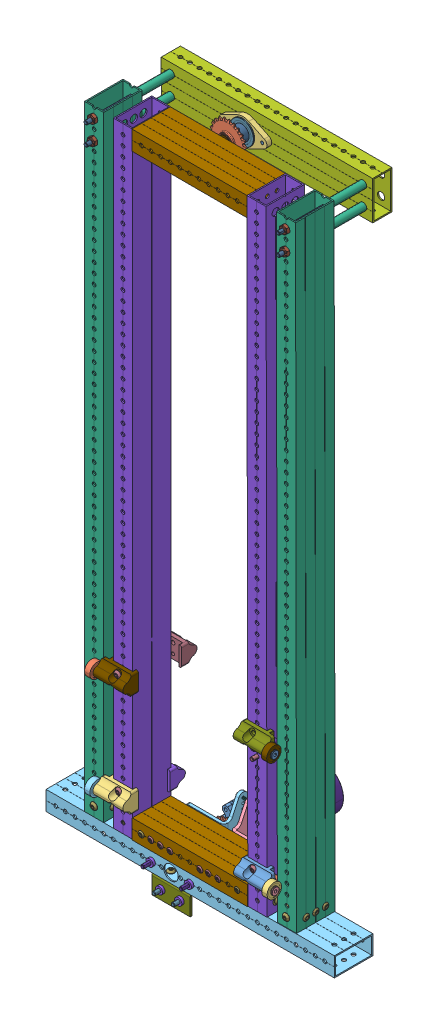
SolidWorks assembly WCP - GreyT Elevator (Cascade, 1 Stage).step, configuration Default. Lengths in mm. (continued)
Components (placement in the parent): (continued)
- WCP-0379 Rev1^WCP - GreyT Elevator (Cascade, 1 Stage).step-4: WCP-0379 Rev1^WCP - GreyT Elevator (Cascade, 1 Stage).step [Default] at (-127 22.225 0) x (0 0 -1) z (1 0 0) size (47.24 20.64 21.84) (virtual)
- WCP-0374 Rev1^WCP - GreyT Elevator (Cascade, 1 Stage).step-4: WCP-0374 Rev1^WCP - GreyT Elevator (Cascade, 1 Stage).step [Default] at (-127 22.225 0) x (0 0 -1) z (1 0 0) size (44.07 19.05 18.67) (virtual)
- 10-32 BHCS - No Thread_WCP-0252 - 0.375^WCP - GreyT Elevator (Cascade, 1 Stage).step-30: 10-32 BHCS - No Thread_WCP-0252 - 0.375^WCP - GreyT Elevator (Cascade, 1 Stage).step [Default] at (-127 11.1125 -12.7) x (-0.583861 0 0.811854) z (0.811854 0 0.583861) size (9.17 12.1 9.17) (virtual)
- 10-32 BHCS - No Thread_WCP-0252 - 0.375^WCP - GreyT Elevator (Cascade, 1 Stage).step-31: 10-32 BHCS - No Thread_WCP-0252 - 0.375^WCP - GreyT Elevator (Cascade, 1 Stage).step [Default] at (-127 11.1125 0) x (-0.583861 0 0.811854) z (0.811854 0 0.583861) size (9.17 12.1 9.17) (virtual)
- 10-32 BHCS - No Thread_WCP-0252 - 0.375^WCP - GreyT Elevator (Cascade, 1 Stage).step-32: 10-32 BHCS - No Thread_WCP-0252 - 0.375^WCP - GreyT Elevator (Cascade, 1 Stage).step [Default] at (-127 11.1125 12.7) x (-0.583861 0 0.811854) z (0.811854 0 0.583861) size (9.17 12.1 9.17) (virtual)
- WCP-0207 Rev1^WCP - GreyT Elevator (Cascade, 1 Stage).step-3: WCP-0207 Rev1^WCP - GreyT Elevator (Cascade, 1 Stage).step [Default] at (-127 812.8 -50.5828) x (0 0 -1) z (0.999873 0.015939 0) size (50.8 9.5 9.5) (virtual)
- WCP-0207 Rev1^WCP - GreyT Elevator (Cascade, 1 Stage).step-4: WCP-0207 Rev1^WCP - GreyT Elevator (Cascade, 1 Stage).step [Default] at (-126.9354 787.4001 -50.5828) x (0 0 -1) z (0.999873 0.015939 0) size (50.8 9.5 9.5) (virtual)
- 10-32 BHCS - No Thread_WCP-0252 - 0.375^WCP - GreyT Elevator (Cascade, 1 Stage).step-33: 10-32 BHCS - No Thread_WCP-0252 - 0.375^WCP - GreyT Elevator (Cascade, 1 Stage).step [Default] at (-127 25.4 25.4) x (-0.238233 -0.971208 0) z (-0.971208 0.238233 0) size (9.17 12.1 9.17) (virtual)
- 10-32 BHCS - No Thread_WCP-0252 - 0.375^WCP - GreyT Elevator (Cascade, 1 Stage).step-34: 10-32 BHCS - No Thread_WCP-0252 - 0.375^WCP - GreyT Elevator (Cascade, 1 Stage).step [Default] at (-127 25.4 -25.4) x (-0.705419 -0.708791 0) z (0.708791 -0.705419 0) size (9.17 12.1 9.17) (virtual)
- WCP-EX-0018-003^WCP - GreyT Elevator (Cascade, 1 Stage).step-2: WCP-EX-0018-003^WCP - GreyT Elevator (Cascade, 1 Stage).step [Default] at (-88.9 127 0) x (0 1 0) z (1 0 0) size (812.8 50.8 25.4) (virtual)
- 10-32 BHCS - No Thread_WCP-0261 - 2.500^WCP - GreyT Elevator (Cascade, 1 Stage).step-11: 10-32 BHCS - No Thread_WCP-0261 - 2.500^WCP - GreyT Elevator (Cascade, 1 Stage).step [Default] at (-88.9 63.5 30.1625) x (-0.238233 -0.971208 0) z (-0.971208 0.238233 0) size (9.17 66.07 9.17) (virtual)
- 10-32 BHCS - No Thread_WCP-0261 - 2.500^WCP - GreyT Elevator (Cascade, 1 Stage).step-12: 10-32 BHCS - No Thread_WCP-0261 - 2.500^WCP - GreyT Elevator (Cascade, 1 Stage).step [Default] at (-88.9 50.8 -30.1625) x (-0.035589 0.999367 0) z (-0.999367 -0.035589 0) size (9.17 66.07 9.17) (virtual)
- 10-32 BHCS - No Thread_WCP-0261 - 2.500^WCP - GreyT Elevator (Cascade, 1 Stage).step-13: 10-32 BHCS - No Thread_WCP-0261 - 2.500^WCP - GreyT Elevator (Cascade, 1 Stage).step [Default] at (-88.8365 198.4231 32.0651) x (-0.238233 -0.971208 0) z (-0.971208 0.238233 0) size (9.17 66.07 9.17) (virtual)
- 10-32 BHCS - No Thread_WCP-0261 - 2.500^WCP - GreyT Elevator (Cascade, 1 Stage).step-14: 10-32 BHCS - No Thread_WCP-0261 - 2.500^WCP - GreyT Elevator (Cascade, 1 Stage).step [Default] at (-88.8365 185.7231 -30.1625) x (-0.035589 0.999367 0) z (-0.999367 -0.035589 0) size (9.17 66.07 9.17) (virtual)
- 10-32 BHCS - No Thread_WCP-0252 - 0.375^WCP - GreyT Elevator (Cascade, 1 Stage).step-35: 10-32 BHCS - No Thread_WCP-0252 - 0.375^WCP - GreyT Elevator (Cascade, 1 Stage).step [Default] at (-77.7875 25.4 -12.7) x (0 0.635714 0.771925) z (0 -0.771925 0.635714) size (9.17 12.1 9.17) (virtual)
- 10-32 BHCS - No Thread_WCP-0252 - 0.375^WCP - GreyT Elevator (Cascade, 1 Stage).step-36: 10-32 BHCS - No Thread_WCP-0252 - 0.375^WCP - GreyT Elevator (Cascade, 1 Stage).step [Default] at (-77.7875 25.4 0) x (0 0.635714 0.771925) z (0 -0.771925 0.635714) size (9.17 12.1 9.17) (virtual)
- 10-32 BHCS - No Thread_WCP-0252 - 0.375^WCP - GreyT Elevator (Cascade, 1 Stage).step-37: 10-32 BHCS - No Thread_WCP-0252 - 0.375^WCP - GreyT Elevator (Cascade, 1 Stage).step [Default] at (-77.7875 25.4 12.7) x (0 0.635714 0.771925) z (0 -0.771925 0.635714) size (9.17 12.1 9.17) (virtual)
- 10-32 BHCS - No Thread_WCP-0252 - 0.375^WCP - GreyT Elevator (Cascade, 1 Stage).step-38: 10-32 BHCS - No Thread_WCP-0252 - 0.375^WCP - GreyT Elevator (Cascade, 1 Stage).step [Default] at (-63.5 25.4 25.4) x (-0.238233 -0.971208 0) z (-0.971208 0.238233 0) size (9.17 12.1 9.17) (virtual)
- WCP-0374 Rev1^WCP - GreyT Elevator (Cascade, 1 Stage).step-5: WCP-0374 Rev1^WCP - GreyT Elevator (Cascade, 1 Stage).step [Default] at (-66.675 25.4 0) x (0 0 -1) z (0 -1 0) size (44.07 19.05 18.67) (virtual)
- WCP-0379 Rev1^WCP - GreyT Elevator (Cascade, 1 Stage).step-5: WCP-0379 Rev1^WCP - GreyT Elevator (Cascade, 1 Stage).step [Default] at (-66.675 25.4 0) x (0 0 -1) z (0 -1 0) size (47.24 20.64 21.84) (virtual)
- 10-32 BHCS - No Thread_WCP-0252 - 0.375^WCP - GreyT Elevator (Cascade, 1 Stage).step-39: 10-32 BHCS - No Thread_WCP-0252 - 0.375^WCP - GreyT Elevator (Cascade, 1 Stage).step [Default] at (-63.5 25.4 -25.4) x (-0.705419 -0.708791 0) z (0.708791 -0.705419 0) size (9.17 12.1 9.17) (virtual)
- 10-32 BHCS - No Thread_WCP-0252 - 0.375^WCP - GreyT Elevator (Cascade, 1 Stage).step-40: 10-32 BHCS - No Thread_WCP-0252 - 0.375^WCP - GreyT Elevator (Cascade, 1 Stage).step [Default] at (-88.7441 24.976 -25.2488) x (-0.705419 -0.708791 0) z (0.708791 -0.705419 0) size (9.17 12.1 9.17) (virtual)
- 10-32 BHCS - No Thread_WCP-0252 - 0.375^WCP - GreyT Elevator (Cascade, 1 Stage).step-41: 10-32 BHCS - No Thread_WCP-0252 - 0.375^WCP - GreyT Elevator (Cascade, 1 Stage).step [Default] at (-72.5907 24.976 -1.6268) x (0 0.635714 0.771925) z (0 -0.771925 0.635714) size (9.17 12.1 9.17) (virtual)
- 10-32 BHCS - No Thread_WCP-0252 - 0.375^WCP - GreyT Elevator (Cascade, 1 Stage).step-42: 10-32 BHCS - No Thread_WCP-0252 - 0.375^WCP - GreyT Elevator (Cascade, 1 Stage).step [Default] at (-72.5907 24.976 11.0732) x (0 0.635714 0.771925) z (0 -0.771925 0.635714) size (9.17 12.1 9.17) (virtual)
- 10-32 BHCS - No Thread_WCP-0252 - 0.375^WCP - GreyT Elevator (Cascade, 1 Stage).step-43: 10-32 BHCS - No Thread_WCP-0252 - 0.375^WCP - GreyT Elevator (Cascade, 1 Stage).step [Default] at (-72.4033 24.976 -14.3268) x (0 0.635714 0.771925) z (0 -0.771925 0.635714) size (9.17 12.1 9.17) (virtual)
- 10-32 BHCS - No Thread_WCP-0252 - 0.375^WCP - GreyT Elevator (Cascade, 1 Stage).step-44: 10-32 BHCS - No Thread_WCP-0252 - 0.375^WCP - GreyT Elevator (Cascade, 1 Stage).step [Default] at (-88.7441 24.976 21.9952) x (-0.238233 -0.971208 0) z (-0.971208 0.238233 0) size (9.17 12.1 9.17) (virtual)
- WCP-0379 Rev1^WCP - GreyT Elevator (Cascade, 1 Stage).step-6: WCP-0379 Rev1^WCP - GreyT Elevator (Cascade, 1 Stage).step [Default] at (-91.9191 24.849 -1.6268) x (0 0 -1) z (0 -1 0) size (47.24 20.64 21.84) (virtual)
- WCP-0374 Rev1^WCP - GreyT Elevator (Cascade, 1 Stage).step-6: WCP-0374 Rev1^WCP - GreyT Elevator (Cascade, 1 Stage).step [Default] at (-91.9191 24.976 -1.6268) x (0 0 -1) z (0 -1 0) size (44.07 19.05 18.67) (virtual)
- WCP-0583-027 Rev1^WCP - GreyT Elevator (Cascade, 1 Stage).step-1: WCP-0583-027 Rev1^WCP - GreyT Elevator (Cascade, 1 Stage).step [Default] at (-38.1 -12.7 25.4) x (0 -1 0) z (1 0 0) size (25.4 25.4 50.8) (virtual)
- REV-21-1650-V1.1.step-1: REV-21-1650-V1.1.step [Default] at (-25.4 0 -115.5875) size (68.13 68.01 93.35)
- REV-21-2102-4-1-cartridge-1: REV-21-2102-4-1-cartridge [Default] at (-25.4 0 -90.2375) size (61.91 50.8 16.85)
- REV-21-2104-hex-socket-output-1: REV-21-2104-hex-socket-output [Default] at (-25.4 0 -74.4125) x (0 0 1) z (-1 0 0) size (23.2 50.8 61.92)
- REV-21-2106-universal-input-1: REV-21-2106-universal-input [Default] at (-25.4 0 -106.0625) size (61.91 50.8 19.05)
- 1_500_L_10_thru_WCP-0205-2: 1_500_L_10_thru_WCP-0205 [Default] at (12.7 0 -43.561) x (0 0 1) z (-0.94684 -0.321705 0) size (38.1 9.5 9.5)
- 1_500_L_10_thru_WCP-0205-3: 1_500_L_10_thru_WCP-0205 [Default] at (-63.5 0 -43.561) x (0 0 1) z (-0.860119 0.510093 0) size (38.1 9.5 9.5)
- Part4^WCP - GreyT Elevator (Cascade, 1 Stage).step-1: Part4^WCP - GreyT Elevator (Cascade, 1 Stage).step [Default] at (-25.4 0 -64.8875) (virtual)
Mates (geometry in assembly coordinates):
- Coincident1: coincident aligned: plane of WCP-EX-0018-005^WCP - GreyT Elevator (Cascade, 1 Stage).step-1 through (126.705 826.1491 0.0759) normal (-0.001569 0.999999 0.000005); plane of WCP-EX-0018-003^WCP - GreyT Elevator (Cascade, 1 Stage).step-1 through (88.6027 826.0894 1.0044) normal (-0.001569 0.999999 0.000005)
- Distance2: distance = 12.7 mm anti-aligned: plane of WCP-EX-0018-003^WCP - GreyT Elevator (Cascade, 1 Stage).step-1 through (101.7227 597.5098 -24.3659) normal (0.999996 0.001569 0.002419); plane of WCP-EX-0018-005^WCP - GreyT Elevator (Cascade, 1 Stage).step-1 through (115.2188 13.33 25.4412) normal (-0.999996 -0.001569 -0.002419)
- Coincident13: coincident anti-aligned: plane of WCP-EX-0018-002^WCP - GreyT Elevator (Cascade, 1 Stage).step-1 through (139.796 775.3781 -75.9828) normal (0 0 1); circle of WCP-0207 Rev1^WCP - GreyT Elevator (Cascade, 1 Stage).step-3
- Distance9: distance = 6.3627 mm aligned: plane of WCP-0326 Rev1^WCP - GreyT Elevator (Cascade, 1 Stage).step-12 through (-126.9354 787.4001 30.367) normal (0 0 1); plane of 10-32 SHCS - No Thread_WCP-0274 - 4.500^WCP - GreyT Elevator (Cascade, 1 Stage).step-4 through (-126.9354 787.4001 36.7297) normal (0 0 1)
- Distance10: distance = 6.3627 mm aligned: plane of WCP-0326 Rev1^WCP - GreyT Elevator (Cascade, 1 Stage).step-2 through (126.9992 813.4457 30.367) normal (0 0 1); plane of 10-32 SHCS - No Thread_WCP-0274 - 4.500^WCP - GreyT Elevator (Cascade, 1 Stage).step-2 through (126.9992 813.4457 36.7297) normal (0 0 1)
- Distance11: distance = 6.3627 mm aligned: plane of WCP-0326 Rev1^WCP - GreyT Elevator (Cascade, 1 Stage).step-1 through (127.0637 788.0458 30.367) normal (0 0 1); plane of 10-32 SHCS - No Thread_WCP-0274 - 4.500^WCP - GreyT Elevator (Cascade, 1 Stage).step-1 through (127.0637 788.0458 36.7297) normal (0 0 1)
- Concentric2: concentric anti-aligned: circle of WCP-0326 Rev1^WCP - GreyT Elevator (Cascade, 1 Stage).step-12; circle of 10-32 SHCS - No Thread_WCP-0274 - 4.500^WCP - GreyT Elevator (Cascade, 1 Stage).step-4
- Concentric4: concentric anti-aligned: circle of 10-32 SHCS - No Thread_WCP-0274 - 4.500^WCP - GreyT Elevator (Cascade, 1 Stage).step-2; circle of WCP-0326 Rev1^WCP - GreyT Elevator (Cascade, 1 Stage).step-2
- Concentric5: concentric anti-aligned: circle of WCP-0326 Rev1^WCP - GreyT Elevator (Cascade, 1 Stage).step-11; circle of 10-32 SHCS - No Thread_WCP-0274 - 4.500^WCP - GreyT Elevator (Cascade, 1 Stage).step-3
- Concentric9: concentric anti-aligned: cylinder of 10-32 SHCS - No Thread_WCP-0274 - 4.500^WCP - GreyT Elevator (Cascade, 1 Stage).step-3 through (-127 812.8 36.7297) axis (0 0 -1) radius 2.413; cylinder of WCP-0207 Rev1^WCP - GreyT Elevator (Cascade, 1 Stage).step-3 through (-127 812.8 -75.9828) axis (0 0 1) radius 2.4892
- Concentric10: concentric anti-aligned: cylinder of 10-32 SHCS - No Thread_WCP-0274 - 4.500^WCP - GreyT Elevator (Cascade, 1 Stage).step-4 through (-126.9354 787.4001 36.7297) axis (0 0 -1) radius 2.413; cylinder of WCP-0207 Rev1^WCP - GreyT Elevator (Cascade, 1 Stage).step-4 through (-126.9354 787.4001 -75.9828) axis (0 0 1) radius 2.4892
- Concentric11: concentric anti-aligned: cylinder of 10-32 SHCS - No Thread_WCP-0274 - 4.500^WCP - GreyT Elevator (Cascade, 1 Stage).step-2 through (126.9992 813.4457 36.7297) axis (0 0 -1) radius 2.413; cylinder of WCP-0207 Rev1^WCP - GreyT Elevator (Cascade, 1 Stage).step-1 through (126.9992 813.4457 -75.9828) axis (0 0 1) radius 2.4892
- Concentric12: concentric anti-aligned: cylinder of 10-32 SHCS - No Thread_WCP-0274 - 4.500^WCP - GreyT Elevator (Cascade, 1 Stage).step-1 through (127.0637 788.0458 36.7297) axis (0 0 -1) radius 2.413; cylinder of WCP-0207 Rev1^WCP - GreyT Elevator (Cascade, 1 Stage).step-2 through (127.0637 788.0458 -75.9828) axis (0 0 1) radius 2.4892
- Concentric13: concentric aligned: circle of 10-32 SHCS - No Thread_WCP-0274 - 4.500^WCP - GreyT Elevator (Cascade, 1 Stage).step-1; circle of WCP-0326 Rev1^WCP - GreyT Elevator (Cascade, 1 Stage).step-1
- Concentric14: concentric anti-aligned: circle of WCP-EX-0018-002^WCP - GreyT Elevator (Cascade, 1 Stage).step-1; circle of WCP-0207 Rev1^WCP - GreyT Elevator (Cascade, 1 Stage).step-4
- Concentric15: concentric anti-aligned: circle of WCP-EX-0018-002^WCP - GreyT Elevator (Cascade, 1 Stage).step-1; circle of WCP-0207 Rev1^WCP - GreyT Elevator (Cascade, 1 Stage).step-2
- Concentric16: concentric anti-aligned: circle of WCP-EX-0018-002^WCP - GreyT Elevator (Cascade, 1 Stage).step-1; circle of WCP-0207 Rev1^WCP - GreyT Elevator (Cascade, 1 Stage).step-1
- Concentric17: concentric anti-aligned: circle of WCP-EX-0018-002^WCP - GreyT Elevator (Cascade, 1 Stage).step-1; circle of WCP-0207 Rev1^WCP - GreyT Elevator (Cascade, 1 Stage).step-3
- Concentric18: concentric anti-aligned: cylinder of 10-32 BHCS - No Thread_WCP-0257 - 1.500.step-1 through (0.0319 800.4229 -69.6328) axis (0 0 -1) radius 2.3749; cylinder of WCP-0476 Rev1^WCP - GreyT Elevator (Cascade, 1 Stage).step-2 through (0.0319 800.4229 -69.6328) axis (0 0 1) radius 2.0193
- Concentric19: concentric anti-aligned: cylinder of 10-32 BHCS - No Thread_WCP-0257 - 1.500.step-2 through (-50.768 800.2938 -69.6328) axis (0 0 -1) radius 2.3749; cylinder of WCP-0476 Rev1^WCP - GreyT Elevator (Cascade, 1 Stage).step-2 through (-50.768 800.2938 -69.6328) axis (0 0 1) radius 2.0193
- Concentric20: concentric anti-aligned: cylinder of 10-32 BHCS - No Thread_WCP-0257 - 1.500.step-2 through (-50.768 800.2938 -69.6328) axis (0 0 -1) radius 2.3749; cylinder of WCP-0476 Rev1^WCP - GreyT Elevator (Cascade, 1 Stage).step-3 through (-50.768 800.2938 -101.3828) axis (0 0 1) radius 2.0193
- Coincident38: coincident anti-aligned: plane of 10-32 BHCS - No Thread_WCP-0257 - 1.500.step-1 through (0.0319 800.4229 -107.7328) normal (0 0 1); plane of WCP-0476 Rev1^WCP - GreyT Elevator (Cascade, 1 Stage).step-3 through (-25.368 800.2938 -107.7328) normal (0 0 -1)
- Coincident39: coincident anti-aligned: plane of 10-32 BHCS - No Thread_WCP-0257 - 1.500.step-2 through (-50.768 800.2938 -107.7328) normal (0 0 1); plane of WCP-0476 Rev1^WCP - GreyT Elevator (Cascade, 1 Stage).step-3 through (-25.368 800.2938 -107.7328) normal (0 0 -1)
- Concentric24: concentric anti-aligned: cylinder of WCP-EX-0018-002^WCP - GreyT Elevator (Cascade, 1 Stage).step-1 through (126.9992 813.4457 -75.9818) axis (0 0 -1) radius 4.7625; cylinder of WCP-0207 Rev1^WCP - GreyT Elevator (Cascade, 1 Stage).step-1 through (126.9992 813.4457 -75.9828) axis (0 0 1) radius 4.7498
- Concentric25: concentric anti-aligned: cylinder of WCP-EX-0018-002^WCP - GreyT Elevator (Cascade, 1 Stage).step-1 through (127.0637 788.0458 -75.9818) axis (0 0 -1) radius 4.7625; cylinder of WCP-0207 Rev1^WCP - GreyT Elevator (Cascade, 1 Stage).step-2 through (127.0637 788.0458 -75.9828) axis (0 0 1) radius 4.7498
- Coincident41: coincident anti-aligned: plane of WCP-EX-0018-002^WCP - GreyT Elevator (Cascade, 1 Stage).step-1 through (139.796 775.3781 -75.9828) normal (0 0 1); plane of WCP-0207 Rev1^WCP - GreyT Elevator (Cascade, 1 Stage).step-2 through (127.0637 788.0458 -75.9828) normal (0 0 -1)
- Coincident42: coincident anti-aligned: plane of WCP-EX-0018-002^WCP - GreyT Elevator (Cascade, 1 Stage).step-1 through (139.796 775.3781 -75.9828) normal (0 0 1); plane of WCP-0207 Rev1^WCP - GreyT Elevator (Cascade, 1 Stage).step-1 through (126.9992 813.4457 -75.9828) normal (0 0 -1)
- Coincident43: coincident anti-aligned: plane of WCP-EX-0018-002^WCP - GreyT Elevator (Cascade, 1 Stage).step-1 through (139.7314 800.778 -77.5703) normal (0 0 -1); plane of 10-32 SHCS - No Thread_WCP-0274 - 4.500^WCP - GreyT Elevator (Cascade, 1 Stage).step-4 through (-126.9354 787.4001 -77.5703) normal (0 0 1)
- Concentric26: concentric anti-aligned: cylinder of WCP-0476 Rev1^WCP - GreyT Elevator (Cascade, 1 Stage).step-2 through (-25.368 800.3583 -69.6328) axis (0 0 -1) radius 14.2875; cylinder of WCP-0785_0_500_flanged_thunderhex_bearing.step-3 through (-25.368 800.3583 -18.7651) axis (0 0 1) radius 14.2875
- Concentric27: concentric aligned: circle of WCP-0790_500L_500_hex.step-1; cylinder of WCP-0785_0_500_flanged_thunderhex_bearing.step-3 through (-25.368 800.3583 -18.7651) axis (0 0 1) radius 6.875
- Coincident44: coincident anti-aligned: plane of WCP-0599 Rev1^WCP - GreyT Elevator (Cascade, 1 Stage).step-1 through (-26.1223 793.9249 -109.3203) normal (-0.128795 -0.991671 0); plane of WCP-0790_500L_500_hex.step-1 through (-29.9106 794.4169 -55.3453) normal (0.128795 0.991671 0)
- Coincident45: coincident anti-aligned: plane of WCP-0599 Rev1^WCP - GreyT Elevator (Cascade, 1 Stage).step-1 through (-20.2716 796.3603 -109.3203) normal (0.794415 -0.607376 0); plane of WCP-0790_500L_500_hex.step-1 through (-22.4939 793.4536 -55.3453) normal (-0.794415 0.607376 0)
- Coincident46: coincident anti-aligned: plane of WCP-0560 Rev1^WCP - GreyT Elevator (Cascade, 1 Stage).step-2 through (-22.4939 793.4536 -45.8203) normal (0.128795 0.991671 0); plane of WCP-0599 Rev1^WCP - GreyT Elevator (Cascade, 1 Stage).step-1 through (-26.1223 793.9249 -109.3203) normal (-0.128795 -0.991671 0)
- Coincident47: coincident anti-aligned: plane of WCP-0560 Rev1^WCP - GreyT Elevator (Cascade, 1 Stage).step-2 through (-18.0226 799.3019 -45.8203) normal (-0.794415 0.607376 0); plane of WCP-0599 Rev1^WCP - GreyT Elevator (Cascade, 1 Stage).step-1 through (-20.2716 796.3603 -109.3203) normal (0.794415 -0.607376 0)
- Concentric28: concentric anti-aligned: circle of WCP-0571 Rev1^WCP - GreyT Elevator (Cascade, 1 Stage).step-1; circle of WCP-0599 Rev1^WCP - GreyT Elevator (Cascade, 1 Stage).step-1
- Coincident49: coincident aligned: plane of WCP-0560 Rev1^WCP - GreyT Elevator (Cascade, 1 Stage).step-2 through (-25.323 800.25 -45.8203) normal (0 0 1); plane of WCP-0599 Rev1^WCP - GreyT Elevator (Cascade, 1 Stage).step-1 through (-25.3061 800.2094 -45.8203) normal (0 0 1)
- Coincident50: coincident anti-aligned: plane of WCP-0571 Rev1^WCP - GreyT Elevator (Cascade, 1 Stage).step-1 through (-25.3061 795.6247 -45.8203) normal (0 0 -1); plane of WCP-0560 Rev1^WCP - GreyT Elevator (Cascade, 1 Stage).step-2 through (-25.323 800.25 -45.8203) normal (0 0 1)
- Concentric29: concentric anti-aligned: cylinder of WCP-EX-0018-002^WCP - GreyT Elevator (Cascade, 1 Stage).step-1 through (-50.768 800.2938 -75.9828) axis (0 0 -1) radius 2.4892; cylinder of WCP-0476 Rev1^WCP - GreyT Elevator (Cascade, 1 Stage).step-2 through (-50.768 800.2938 -69.6328) axis (0 0 1) radius 2.0193
- Concentric30: concentric anti-aligned: cylinder of WCP-EX-0018-002^WCP - GreyT Elevator (Cascade, 1 Stage).step-1 through (0.0319 800.4229 -75.9828) axis (0 0 -1) radius 2.4892; cylinder of WCP-0476 Rev1^WCP - GreyT Elevator (Cascade, 1 Stage).step-2 through (0.0319 800.4229 -69.6328) axis (0 0 1) radius 2.0193
- Coincident51: coincident anti-aligned: plane of WCP-0560 Rev1^WCP - GreyT Elevator (Cascade, 1 Stage).step-2 through (-25.323 800.25 -55.3453) normal (0 0 -1); plane of WCP-0790_500L_500_hex.step-1 through (-25.368 800.3583 -55.3453) normal (0 0 1)
- Concentric31: concentric aligned: circle of WCP-0571 Rev1^WCP - GreyT Elevator (Cascade, 1 Stage).step-2; circle of WCP-0599 Rev1^WCP - GreyT Elevator (Cascade, 1 Stage).step-1
- Concentric32: concentric anti-aligned: circle of WCP-0476 Rev1^WCP - GreyT Elevator (Cascade, 1 Stage).step-3; circle of WCP-0785_0_500_flanged_thunderhex_bearing.step-2
- Coincident55: coincident anti-aligned: plane of WCP-0476 Rev1^WCP - GreyT Elevator (Cascade, 1 Stage).step-2 through (-25.368 800.3583 -69.6328) normal (0 0 1); plane of WCP-0785_0_500_flanged_thunderhex_bearing.step-3 through (-36.1398 809.7445 -69.6328) normal (0 0 -1)
- Coincident56: coincident anti-aligned: plane of WCP-0790_500L_500_hex.step-1 through (-25.368 800.3583 -68.0453) normal (0 0 -1); plane of WCP-0785_0_500_flanged_thunderhex_bearing.step-3 through (-32.6073 806.6664 -68.0453) normal (0 0 1)
- Coincident57: coincident anti-aligned: plane of WCP-EX-0018-002^WCP - GreyT Elevator (Cascade, 1 Stage).step-1 through (139.796 775.3781 -75.9828) normal (0 0 1); plane of WCP-0476 Rev1^WCP - GreyT Elevator (Cascade, 1 Stage).step-2 through (-25.368 800.3583 -75.9828) normal (0 0 -1)
- Coincident58: coincident anti-aligned: plane of WCP-EX-0018-002^WCP - GreyT Elevator (Cascade, 1 Stage).step-1 through (139.796 775.3781 -101.3828) normal (0 0 -1); plane of WCP-0476 Rev1^WCP - GreyT Elevator (Cascade, 1 Stage).step-3 through (-25.368 800.2938 -101.3828) normal (0 0 1)
- Coincident59: coincident anti-aligned: plane of WCP-0476 Rev1^WCP - GreyT Elevator (Cascade, 1 Stage).step-3 through (-25.368 800.2938 -107.7328) normal (0 0 -1); plane of WCP-0785_0_500_flanged_thunderhex_bearing.step-2 through (-19.5771 813.3551 -107.7328) normal (0 0 1)
- Coincident60: coincident anti-aligned: plane of WCP-0571 Rev1^WCP - GreyT Elevator (Cascade, 1 Stage).step-2 through (-24.6727 795.6687 -109.3203) normal (0 0 1); plane of WCP-0599 Rev1^WCP - GreyT Elevator (Cascade, 1 Stage).step-1 through (-25.3061 800.2094 -109.3203) normal (0 0 -1)
- Distance12: distance = 6.5799 mm aligned: plane of WCP-0326 Rev1^WCP - GreyT Elevator (Cascade, 1 Stage).step-11 through (-127 812.8 30.1498) normal (0 0 1); plane of 10-32 SHCS - No Thread_WCP-0274 - 4.500^WCP - GreyT Elevator (Cascade, 1 Stage).step-3 through (-127 812.8 36.7297) normal (0 0 1)
- Coincident69: coincident anti-aligned: plane of WCP-EX-0018-002^WCP - GreyT Elevator (Cascade, 1 Stage).step-1 through (139.796 775.3781 -75.9828) normal (0 0 1); plane of WCP-0207 Rev1^WCP - GreyT Elevator (Cascade, 1 Stage).step-4 through (-126.9354 787.4001 -75.9828) normal (0 0 -1)
- Coincident70: coincident anti-aligned: plane of WCP-EX-0018-002^WCP - GreyT Elevator (Cascade, 1 Stage).step-1 through (139.7314 800.778 -77.5703) normal (0 0 -1); plane of 10-32 SHCS - No Thread_WCP-0274 - 4.500^WCP - GreyT Elevator (Cascade, 1 Stage).step-3 through (-127 812.8 -77.5703) normal (0 0 1)
- Coincident71: coincident aligned: plane of 10-32 SHCS - No Thread_WCP-0274 - 4.500^WCP - GreyT Elevator (Cascade, 1 Stage).step-1 through (127.0637 788.0458 36.7297) normal (0 0 1); plane of 10-32 SHCS - No Thread_WCP-0274 - 4.500^WCP - GreyT Elevator (Cascade, 1 Stage).step-2 through (126.9992 813.4457 36.7297) normal (0 0 1)
- Coincident72: coincident aligned: plane of 10-32 SHCS - No Thread_WCP-0274 - 4.500^WCP - GreyT Elevator (Cascade, 1 Stage).step-3 through (-127 812.8 36.7297) normal (0 0 1); plane of 10-32 SHCS - No Thread_WCP-0274 - 4.500^WCP - GreyT Elevator (Cascade, 1 Stage).step-4 through (-126.9354 787.4001 36.7297) normal (0 0 1)
- Coincident80: coincident anti-aligned: plane of WCP-EX-0018-005^WCP - GreyT Elevator (Cascade, 1 Stage).step-2 through (-114.3 12.7 25.4) normal (0 0 1); plane of WCP-0326 Rev1^WCP - GreyT Elevator (Cascade, 1 Stage).step-11 through (-127 812.8 25.4) normal (0 0 -1)
- Concentric33: concentric aligned: circle of WCP-EX-0018-005^WCP - GreyT Elevator (Cascade, 1 Stage).step-2; circle of 10-32 SHCS - No Thread_WCP-0274 - 4.500^WCP - GreyT Elevator (Cascade, 1 Stage).step-3
- Coincident81: coincident anti-aligned: plane of WCP-EX-0018-003^WCP - GreyT Elevator (Cascade, 1 Stage).step-1 through (76.3228 597.4699 -24.4273) normal (-0.999996 -0.001569 -0.002419); plane of WCP-EX-0018-004^WCP - GreyT Elevator (Cascade, 1 Stage).step-2 through (75.9226 813.3695 0.9736) normal (0.999996 0.001569 0.002419)
- Coincident82: coincident aligned: plane of WCP-EX-0018-003^WCP - GreyT Elevator (Cascade, 1 Stage).step-1 through (88.6027 826.0894 1.0044) normal (-0.001569 0.999999 0.000005); plane of WCP-EX-0018-004^WCP - GreyT Elevator (Cascade, 1 Stage).step-2 through (75.8413 826.0692 26.3736) normal (-0.001569 0.999999 0.000005)
- Coincident83: coincident aligned: plane of WCP-EX-0018-003^WCP - GreyT Elevator (Cascade, 1 Stage).step-1 through (76.1999 597.4695 26.3725) normal (-0.002419 -0.000009 0.999997); plane of WCP-EX-0018-004^WCP - GreyT Elevator (Cascade, 1 Stage).step-2 through (75.8413 826.0692 26.3736) normal (-0.002419 -0.000009 0.999997)
- Coincident84: coincident anti-aligned: plane of WCP-0323 - Elevator Clamping Block-7^WCP - GreyT Elevator (Cascade, 1 Stage).step-1/WCP-0323-001 Rev2(6)^WCP-0323 - Elevator Clamping Block-7_WCP - GreyT Elevator (Cascade, 1 Stage).step-1 through (-101.6 192.0731 20.892) normal (1 0 0); plane of WCP-EX-0018-003^WCP - GreyT Elevator (Cascade, 1 Stage).step-2 through (-101.6 241.3 -25.4) normal (-1 0 0)
- Coincident85: coincident anti-aligned: plane of WCP-0323 - Elevator Clamping Block-7^WCP - GreyT Elevator (Cascade, 1 Stage).step-1/WCP-0323-001 Rev2(6)^WCP-0323 - Elevator Clamping Block-7_WCP - GreyT Elevator (Cascade, 1 Stage).step-1 through (-101.6 192.0731 25.4) normal (0 0 -1); plane of WCP-EX-0018-003^WCP - GreyT Elevator (Cascade, 1 Stage).step-2 through (-76.2 241.3 25.4) normal (0 0 1)
- Concentric49: concentric aligned: cylinder of WCP-0323 - Elevator Clamping Block-7^WCP - GreyT Elevator (Cascade, 1 Stage).step-1/WCP-0323-001 Rev2(6)^WCP-0323 - Elevator Clamping Block-7_WCP - GreyT Elevator (Cascade, 1 Stage).step-1 through (-88.8365 185.7231 41.275) axis (0 0 -1) radius 2.4892; cylinder of 10-32 BHCS - No Thread_WCP-0261 - 2.500^WCP - GreyT Elevator (Cascade, 1 Stage).step-14 through (-88.8365 185.7231 33.3375) axis (0 0 -1) radius 2.3749
- Coincident86: coincident aligned: plane of WCP-0323 - Elevator Clamping Block-6^WCP - GreyT Elevator (Cascade, 1 Stage).step-1/WCP-0323-001 Rev2(3)^WCP-0323 - Elevator Clamping Block-6_WCP - GreyT Elevator (Cascade, 1 Stage).step-1 through (-73.025 192.0731 -40.688) normal (1 0 0); plane of WCP-0323 - Elevator Clamping Block-7^WCP - GreyT Elevator (Cascade, 1 Stage).step-1/WCP-0323-001 Rev2(6)^WCP-0323 - Elevator Clamping Block-7_WCP - GreyT Elevator (Cascade, 1 Stage).step-1 through (-73.025 192.0731 25.4) normal (1 0 0)
- Coincident87: coincident aligned: plane of WCP-0323 - Elevator Clamping Block-6^WCP - GreyT Elevator (Cascade, 1 Stage).step-1/WCP-0323-001 Rev2(3)^WCP-0323 - Elevator Clamping Block-6_WCP - GreyT Elevator (Cascade, 1 Stage).step-1 through (-113.5063 204.7731 -40.688) normal (0 1 0); plane of WCP-0323 - Elevator Clamping Block-7^WCP - GreyT Elevator (Cascade, 1 Stage).step-1/WCP-0323-001 Rev2(6)^WCP-0323 - Elevator Clamping Block-7_WCP - GreyT Elevator (Cascade, 1 Stage).step-1 through (-113.5063 204.7731 25.4) normal (0 1 0)
- Concentric51: concentric anti-aligned: cylinder of WCP-0323 - Elevator Clamping Block-7^WCP - GreyT Elevator (Cascade, 1 Stage).step-1/WCP-0323-001 Rev2(6)^WCP-0323 - Elevator Clamping Block-7_WCP - GreyT Elevator (Cascade, 1 Stage).step-1 through (-88.8365 198.4231 41.275) axis (0 0 -1) radius 5.08; circle of 10-32 BHCS - No Thread_WCP-0261 - 2.500^WCP - GreyT Elevator (Cascade, 1 Stage).step-13
- Concentric54: concentric anti-aligned: circle of WCP-0379 Rev1^WCP - GreyT Elevator (Cascade, 1 Stage).step-6; circle of WCP-0374 Rev1^WCP - GreyT Elevator (Cascade, 1 Stage).step-6
- Coincident90: coincident anti-aligned: plane of WCP-0379 Rev1^WCP - GreyT Elevator (Cascade, 1 Stage).step-6 through (-82.3941 34.3105 20.5347) normal (0 -1 0); plane of WCP-0374 Rev1^WCP - GreyT Elevator (Cascade, 1 Stage).step-6 through (-82.3941 34.3105 20.4077) normal (0 1 0)
- Concentric55: concentric anti-aligned: cylinder of 10-32 BHCS - No Thread_WCP-0252 - 0.375^WCP - GreyT Elevator (Cascade, 1 Stage).step-40 through (-88.7441 24.976 -15.7238) axis (0 0 -1) radius 2.3749; cylinder of WCP-0374 Rev1^WCP - GreyT Elevator (Cascade, 1 Stage).step-6 through (-88.7441 24.976 20.4077) axis (0 0 1) radius 2.0193
- Coincident91: coincident anti-aligned: plane of 10-32 BHCS - No Thread_WCP-0252 - 0.375^WCP - GreyT Elevator (Cascade, 1 Stage).step-40 through (-88.7441 24.976 -25.2488) normal (0 0 1); plane of WCP-0379 Rev1^WCP - GreyT Elevator (Cascade, 1 Stage).step-6 through (-82.3941 35.771 -25.2488) normal (0 0 -1)
- Concentric56: concentric anti-aligned: cylinder of 10-32 BHCS - No Thread_WCP-0252 - 0.375^WCP - GreyT Elevator (Cascade, 1 Stage).step-40 through (-88.7441 24.976 -27.8142) axis (0 0 -1) radius 4.5847; cylinder of 10-32 BHCS - No Thread_WCP-0252 - 0.375^WCP - GreyT Elevator (Cascade, 1 Stage).step-44 through (-88.7441 24.976 24.5606) axis (0 0 1) radius 4.5847
- Coincident92: coincident anti-aligned: plane of 10-32 BHCS - No Thread_WCP-0252 - 0.375^WCP - GreyT Elevator (Cascade, 1 Stage).step-44 through (-88.7441 24.976 21.9952) normal (0 0 -1); plane of WCP-0379 Rev1^WCP - GreyT Elevator (Cascade, 1 Stage).step-6 through (-82.3941 35.771 21.9952) normal (0 0 1)
- Concentric58: concentric aligned: cylinder of 10-32 BHCS - No Thread_WCP-0252 - 0.375^WCP - GreyT Elevator (Cascade, 1 Stage).step-43 through (-62.8783 24.976 -14.3268) axis (-1 0 0) radius 2.3749; cylinder of WCP-0374 Rev1^WCP - GreyT Elevator (Cascade, 1 Stage).step-6 through (-101.4441 24.976 -14.3268) axis (-1 0 0) radius 2.0193
- Concentric59: concentric aligned: cylinder of 10-32 BHCS - No Thread_WCP-0252 - 0.375^WCP - GreyT Elevator (Cascade, 1 Stage).step-41 through (-63.0657 24.976 -1.6268) axis (-1 0 0) radius 2.3749; cylinder of WCP-0374 Rev1^WCP - GreyT Elevator (Cascade, 1 Stage).step-6 through (-101.4441 24.976 -1.6268) axis (-1 0 0) radius 2.0193
- Concentric61: concentric aligned: cylinder of 10-32 BHCS - No Thread_WCP-0252 - 0.375^WCP - GreyT Elevator (Cascade, 1 Stage).step-42 through (-63.0657 24.976 11.0732) axis (-1 0 0) radius 2.3749; cylinder of WCP-0374 Rev1^WCP - GreyT Elevator (Cascade, 1 Stage).step-6 through (-101.4441 24.976 11.0732) axis (-1 0 0) radius 2.0193
- Coincident93: coincident anti-aligned: plane of WCP-0323 - Elevator Clamping Block-3^WCP - GreyT Elevator (Cascade, 1 Stage).step-1/WCP-0323-001 Rev2(8)^WCP-0323 - Elevator Clamping Block-3_WCP - GreyT Elevator (Cascade, 1 Stage).step-1 through (102.2013 214.1019 26.4322) normal (0.002419 0.000009 -0.999997); plane of WCP-EX-0018-003^WCP - GreyT Elevator (Cascade, 1 Stage).step-1 through (76.1999 597.4695 26.3725) normal (-0.002419 -0.000009 0.999997)
- Coincident94: coincident anti-aligned: plane of WCP-0323 - Elevator Clamping Block-3^WCP - GreyT Elevator (Cascade, 1 Stage).step-1/WCP-0323-001 Rev2(8)^WCP-0323 - Elevator Clamping Block-3_WCP - GreyT Elevator (Cascade, 1 Stage).step-1 through (102.2123 214.1019 21.9242) normal (-0.999996 -0.001569 -0.002419); plane of WCP-EX-0018-003^WCP - GreyT Elevator (Cascade, 1 Stage).step-1 through (101.7227 597.5098 -24.3659) normal (0.999996 0.001569 0.002419)
- Concentric62: concentric anti-aligned: circle of WCP-0326 Rev1^WCP - GreyT Elevator (Cascade, 1 Stage).step-4; circle of 10-32 BHCS - No Thread_WCP-0261 - 2.500^WCP - GreyT Elevator (Cascade, 1 Stage).step-6
- Coincident97: coincident anti-aligned: plane of #4-40 x .750L SHCS^WCP - GreyT Elevator (Cascade, 1 Stage).step-1 through (5.6113 59.1387 -50.347) normal (-1 0 0); plane of WCP-0583-025 Rev1_DefaultSM-FLAT-PATTERN^WCP - GreyT Elevator (Cascade, 1 Stage).step-1 through (5.6113 17.9189 -30.9875) normal (1 0 0)
- Coincident98: coincident anti-aligned: plane of #4-40 x .750L SHCS^WCP - GreyT Elevator (Cascade, 1 Stage).step-3 through (5.6113 43.9859 -52.7861) normal (-1 0 0); plane of WCP-0583-025 Rev1_DefaultSM-FLAT-PATTERN^WCP - GreyT Elevator (Cascade, 1 Stage).step-1 through (5.6113 17.9189 -30.9875) normal (1 0 0)
- Coincident99: coincident anti-aligned: plane of #4-40 x .750L SHCS^WCP - GreyT Elevator (Cascade, 1 Stage).step-2 through (5.6113 28.7711 -49.9365) normal (-1 0 0); plane of WCP-0583-025 Rev1_DefaultSM-FLAT-PATTERN^WCP - GreyT Elevator (Cascade, 1 Stage).step-1 through (5.6113 17.9189 -30.9875) normal (1 0 0)
- Concentric64: concentric aligned: cylinder of #4-40 x .750L SHCS^WCP - GreyT Elevator (Cascade, 1 Stage).step-2 through (-13.4387 30.6189 -50.8) axis (-1 0 0) radius 2.3241; circle of WCP-0583-025 Rev1_DefaultSM-FLAT-PATTERN^WCP - GreyT Elevator (Cascade, 1 Stage).step-1
- Coincident100: coincident anti-aligned: plane of WCP-0326 Rev1^WCP - GreyT Elevator (Cascade, 1 Stage).step-3 through (38.1 25.4 -29.4) normal (0 0 1); plane of WCP-0583-025 Rev1_DefaultSM-FLAT-PATTERN^WCP - GreyT Elevator (Cascade, 1 Stage).step-1 through (23.8363 24.2689 -29.4) normal (0 0 -1)
- Coincident101: coincident anti-aligned: plane of WCP-0326 Rev1^WCP - GreyT Elevator (Cascade, 1 Stage).step-8 through (25.4 25.4 -29.4) normal (0 0 1); plane of WCP-0583-025 Rev1_DefaultSM-FLAT-PATTERN^WCP - GreyT Elevator (Cascade, 1 Stage).step-1 through (23.8363 24.2689 -29.4) normal (0 0 -1)
- Concentric65: concentric anti-aligned: circle of 10-32 BHCS - No Thread_WCP-0261 - 2.500^WCP - GreyT Elevator (Cascade, 1 Stage).step-1; circle of WCP-0326 Rev1^WCP - GreyT Elevator (Cascade, 1 Stage).step-3
- Concentric66: concentric aligned: circle of WCP-0326 Rev1^WCP - GreyT Elevator (Cascade, 1 Stage).step-8; circle of 10-32 BHCS - No Thread_WCP-0261 - 2.500^WCP - GreyT Elevator (Cascade, 1 Stage).step-5
- Concentric67: concentric aligned: circle of WCP-0326 Rev1^WCP - GreyT Elevator (Cascade, 1 Stage).step-4; circle of 10-32 BHCS - No Thread_WCP-0261 - 2.500^WCP - GreyT Elevator (Cascade, 1 Stage).step-6
- Concentric68: concentric anti-aligned: cylinder of 10-32 BHCS - No Thread_WCP-0261 - 2.500^WCP - GreyT Elevator (Cascade, 1 Stage).step-6 through (14.3113 24.2689 -37.9316) axis (0 0 1) radius 2.3749; cylinder of WCP-0583-025 Rev1_DefaultSM-FLAT-PATTERN^WCP - GreyT Elevator (Cascade, 1 Stage).step-1 through (14.3113 24.2689 -25.4) axis (0 0 -1) radius 2.4892
- Coincident103: coincident anti-aligned: plane of WCP-0326 Rev1^WCP - GreyT Elevator (Cascade, 1 Stage).step-4 through (14.3113 24.2689 -29.4) normal (0 0 1); plane of WCP-0583-025 Rev1_DefaultSM-FLAT-PATTERN^WCP - GreyT Elevator (Cascade, 1 Stage).step-1 through (23.8363 24.2689 -29.4) normal (0 0 -1)
- Coincident106: coincident anti-aligned: plane of WCP-0374 Rev1^WCP - GreyT Elevator (Cascade, 1 Stage).step-3 through (83.4261 35.6035 21.3339) normal (0 1 0); plane of WCP-0379 Rev1^WCP - GreyT Elevator (Cascade, 1 Stage).step-3 through (83.4261 35.6035 21.4609) normal (0 -1 0)
- Concentric70: concentric anti-aligned: circle of WCP-0374 Rev1^WCP - GreyT Elevator (Cascade, 1 Stage).step-3; circle of WCP-0379 Rev1^WCP - GreyT Elevator (Cascade, 1 Stage).step-3
- Concentric71: concentric aligned: cylinder of 10-32 BHCS - No Thread_WCP-0252 - 0.375^WCP - GreyT Elevator (Cascade, 1 Stage).step-20 through (92.9511 26.269 11.9994) axis (1 0 0) radius 2.3749; cylinder of WCP-0374 Rev1^WCP - GreyT Elevator (Cascade, 1 Stage).step-3 through (102.4761 26.269 11.9994) axis (1 0 0) radius 2.0193
- Concentric72: concentric aligned: cylinder of 10-32 BHCS - No Thread_WCP-0252 - 0.375^WCP - GreyT Elevator (Cascade, 1 Stage).step-19 through (92.9511 26.269 -0.7006) axis (1 0 0) radius 2.3749; cylinder of WCP-0374 Rev1^WCP - GreyT Elevator (Cascade, 1 Stage).step-3 through (102.4761 26.269 -0.7006) axis (1 0 0) radius 2.0193
- Concentric73: concentric aligned: cylinder of 10-32 BHCS - No Thread_WCP-0252 - 0.375^WCP - GreyT Elevator (Cascade, 1 Stage).step-21 through (92.9511 26.269 -13.4006) axis (1 0 0) radius 2.3749; cylinder of WCP-0374 Rev1^WCP - GreyT Elevator (Cascade, 1 Stage).step-3 through (102.4761 26.269 -13.4006) axis (1 0 0) radius 2.0193
- Coincident108: coincident aligned: plane of 10-32 BHCS - No Thread_WCP-0252 - 0.375^WCP - GreyT Elevator (Cascade, 1 Stage).step-19 through (105.0415 24.4063 0.8334) normal (1 0 0); plane of 10-32 BHCS - No Thread_WCP-0252 - 0.375^WCP - GreyT Elevator (Cascade, 1 Stage).step-21 through (105.0415 24.4063 -11.8666) normal (1 0 0)
- Coincident109: coincident aligned: plane of 10-32 BHCS - No Thread_WCP-0252 - 0.375^WCP - GreyT Elevator (Cascade, 1 Stage).step-19 through (105.0415 24.4063 0.8334) normal (1 0 0); plane of 10-32 BHCS - No Thread_WCP-0252 - 0.375^WCP - GreyT Elevator (Cascade, 1 Stage).step-20 through (105.0415 24.4063 13.5334) normal (1 0 0)
- Coincident111: coincident anti-aligned: plane of 10-32 BHCS - No Thread_WCP-0252 - 0.375^WCP - GreyT Elevator (Cascade, 1 Stage).step-21 through (102.4761 26.269 -13.4006) normal (-1 0 0); plane of WCP-0374 Rev1^WCP - GreyT Elevator (Cascade, 1 Stage).step-3 through (102.4761 26.269 -0.7006) normal (1 0 0)
- Coincident117: coincident anti-aligned: plane of WCP-EX-0018-003^WCP - GreyT Elevator (Cascade, 1 Stage).step-1 through (76.3228 597.4699 -24.4273) normal (-0.999996 -0.001569 -0.002419); plane of WCP-EX-0018-004^WCP - GreyT Elevator (Cascade, 1 Stage).step-1 through (77.1564 25.867 1.6908) normal (0.999996 0.001569 0.002419)
- Coincident133: coincident anti-aligned: plane of REV-21-1650-V1.1.step-1 through (-25.4 0 -115.5875) normal (0 0 1); plane of REV-21-2106-universal-input-1 through (-25.4 0 -115.5875) normal (0 0 -1)
- Concentric80: concentric anti-aligned: circle of REV-21-1650-V1.1.step-1; circle of REV-21-2106-universal-input-1
- Concentric81: concentric anti-aligned: circle of REV-21-1650-V1.1.step-1; circle of REV-21-2102-4-1-cartridge-1
- Coincident134: coincident anti-aligned: plane of REV-21-2102-4-1-cartridge-1 through (-25.4 0 -96.5375) normal (0 0 -1); plane of REV-21-2106-universal-input-1 through (-25.4 0 -96.5375) normal (0 0 1)
- Concentric82: concentric anti-aligned: circle of REV-21-1650-V1.1.step-1; circle of REV-21-2104-hex-socket-output-1
- Coincident135: coincident anti-aligned: plane of REV-21-2102-4-1-cartridge-1 through (-25.4 0 -83.9375) normal (0 0 1); plane of REV-21-2104-hex-socket-output-1 through (-25.4 0 -83.9375) normal (0 0 -1)
- Concentric85: concentric aligned: circle of WCP-0800_500_hex_collar_high_strength^WCP - GreyT Elevator (Cascade, 1 Stage).step-1; circle of REV-21-2104-hex-socket-output-1
- Coincident136: coincident anti-aligned: plane of WCP-0800_500_hex_collar_high_strength^WCP - GreyT Elevator (Cascade, 1 Stage).step-1 through (-25.4 0 -64.8875) normal (0 0 -1); plane of REV-21-2104-hex-socket-output-1 through (-25.4 0 -64.8875) normal (0 0 1)
- Coincident138: coincident anti-aligned: plane of WCP-EX-0018-001^WCP - GreyT Elevator (Cascade, 1 Stage).step-1 through (190.5 -12.7 -25.4) normal (0 0 -1); plane of 1_500_L_10_thru_WCP-0205-2 through (12.7 0 -25.4) normal (0 0 1)
- Concentric87: concentric aligned: circle of WCP-EX-0018-001^WCP - GreyT Elevator (Cascade, 1 Stage).step-1; circle of 1_500_L_10_thru_WCP-0205-2
- Concentric88: concentric anti-aligned: cylinder of WCP-EX-0018-001^WCP - GreyT Elevator (Cascade, 1 Stage).step-1 through (-63.5 0 -25.4) axis (0 0 1) radius 2.4892; cylinder of 1_500_L_10_thru_WCP-0205-3 through (-63.5 0 -24.511) axis (0 0 -1) radius 4.7498
- Coincident139: coincident anti-aligned: plane of WCP-EX-0018-001^WCP - GreyT Elevator (Cascade, 1 Stage).step-1 through (190.5 -12.7 -25.4) normal (0 0 -1); plane of 1_500_L_10_thru_WCP-0205-3 through (-63.5 0 -25.4) normal (0 0 1)
- Coincident140: coincident anti-aligned: plane of WCP-EX-0018-001^WCP - GreyT Elevator (Cascade, 1 Stage).step-1 through (190.5 -12.7 -25.4) normal (0 0 -1); plane of 1_500_L_10_thru_WCP-0205-3 through (-63.5 0 -25.4) normal (0 0 1)
- Coincident141: coincident anti-aligned: plane of WCP-EX-0018-001^WCP - GreyT Elevator (Cascade, 1 Stage).step-1 through (190.5 -12.7 -25.4) normal (0 0 -1); plane of 1_500_L_10_thru_WCP-0205-2 through (12.7 0 -25.4) normal (0 0 1)
- InPlace2: in place: plane of REV-21-2104-hex-socket-output-1 through (-25.4 0 -64.8875) normal (0 0 1); plane of ? through (0 0 -64.8875) normal (0 0 1); moOrthogonalPlaneRef_w of REV-21-2104-hex-socket-output-1 through (-25.4 0 -64.8875) normal (0 0 1); plane of ? through (0 0 -64.8875) normal (0 1 0); plane of REV-21-2104-hex-socket-output-1 through (-25.4 0 -64.8875) normal (0 0 1); plane of ? through (0 0 -64.8875) normal (1 0 0); plane of REV-21-2104-hex-socket-output-1 through (-25.4 0 -64.8875) normal (0 0 1); unknown of Part4^WCP - GreyT Elevator (Cascade, 1 Stage).step-1
- Coincident142: coincident aligned: plane of REV-21-2104-hex-socket-output-1; plane of Part4^WCP - GreyT Elevator (Cascade, 1 Stage).step-1
- Coincident143: coincident aligned: moOrthogonalPlaneRef_w of REV-21-2104-hex-socket-output-1 through (-25.4 0 -64.8875) normal (0 1 0); plane of Part4^WCP - GreyT Elevator (Cascade, 1 Stage).step-1 through (-25.4 0 -64.8875) normal (0 1 0)
- Coincident144: coincident anti-aligned: moOrthogonalPlaneRef_w of REV-21-2104-hex-socket-output-1 through (-25.4 0 -64.8875) normal (-1 0 0); plane of Part4^WCP - GreyT Elevator (Cascade, 1 Stage).step-1 through (-25.4 0 -64.8875) normal (1 0 0)
